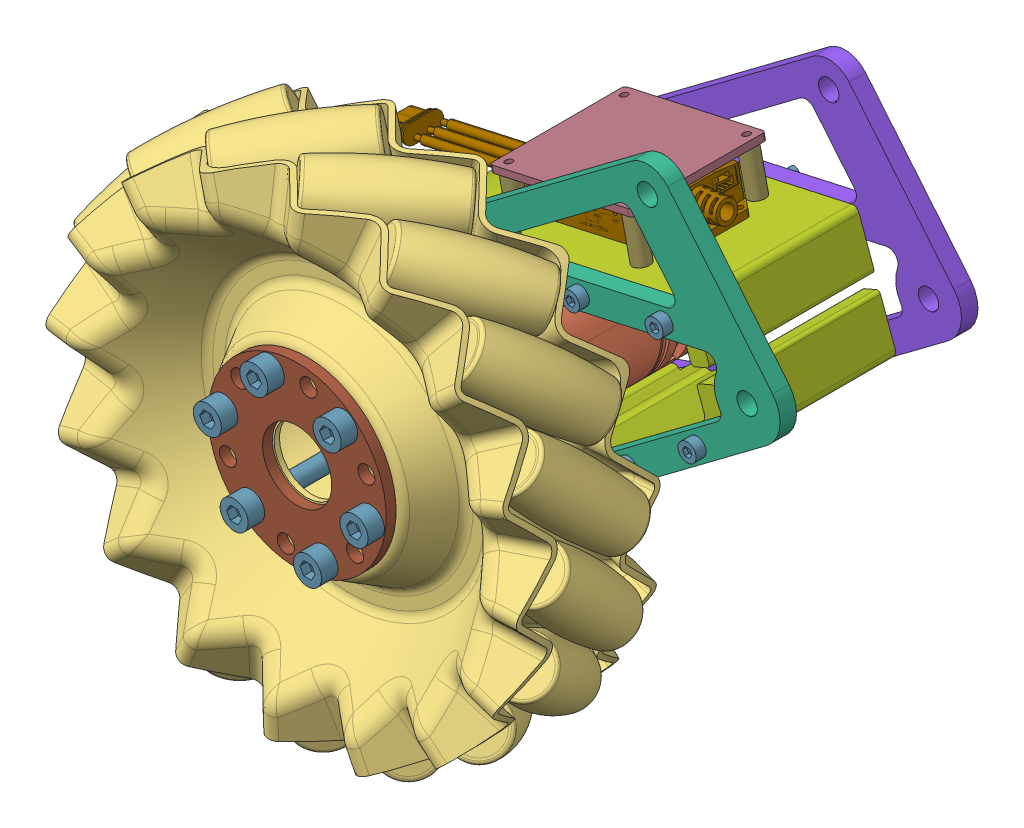
SolidWorks assembly DP_右旋轮组_1, configuration 默认. Lengths in mm.
Overall size (201.98 183.85 131.37).
38 component instances, 14 part files, 81 mates.
Components (placement in the parent):
- DP_夹紧联轴器2-1: DP_夹紧联轴器2 [默认] at (34.8209 73.9788 33.82) x (-0.925598 -0.378508 0) z (0 0 1) size (47.97 54.2 10)
- DP_RoboMaster GM3508无刷减速电机-1: DP_RoboMaster GM3508无刷减速电机 [默认] at origin size (42 44.98 98.4)
- DP_右旋_mecanum_wheel-1: DP_右旋_mecanum_wheel [默认] at (53.3369 61.5614 188.9722) x (0.971628 -0.236514 0) z (0 0 1) size (152.18 152.18 48.1)
- DP_轮组端盖_1-1: DP_轮组端盖_1 [默认] at (34.8209 73.9788 43.82) x (0.996746 -0.080602 0) z (0 0 1) size (19.5 19.5 10)
- DP_10x24x9_推力球轴承-1: DP_10x24x9_推力球轴承 [默认] at (34.8209 73.9788 28.82) x (0.526634 0.850092 0) z (0 0 1) size (24 24 10)
- DP_轮组电机安装板_1-1: DP_轮组电机安装板_1 [默认] at (122.7527 109.937 21.9) x (0.925598 0.378508 0) z (0 0 1) size (139 90.3 5)
- DP_轮组打印件垫块_1-1: DP_轮组打印件垫块_1 [默认] at (122.7527 109.937 -28.1) x (0.925598 0.378508 0) z (0 0 1) size (114.05 68 50)
- DP_轮组电机保护板_1-1: DP_轮组电机保护板_1 [默认] at (122.7527 109.937 -33.1) x (0.925598 0.378508 0) z (0 0 1) size (139 90.3 5)
- DP_C620无刷电机调速器-1: DP_C620无刷电机调速器 [默认] at (56.9242 119.261 -3.1) x (-0.976125 -0.21721 0) z (0 0 1) size (103.05 11.5 26.13)
- DP_滚花铜螺母M2x5-1: DP_滚花铜螺母M2x5 [默认] at (82.9031 114.3875 5.9) x (0.971604 0.216204 0.096132) z (-0.21721 0.976125 0) size (3 3 5)
- DP_滚花铜螺母M2x5-2: DP_滚花铜螺母M2x5 [默认] at (81.817 119.2681 -12.1) x (0.869388 0.193459 0.454684) z (0.21721 -0.976125 0) size (3 3 5)
- DP_滚花铜螺母M2x5-3: DP_滚花铜螺母M2x5 [默认] at (38.7822 104.5696 -12.1) x (0.971604 0.216204 0.096132) z (-0.21721 0.976125 0) size (3 3 5)
- DP_滚花铜螺母M2x5-4: DP_滚花铜螺母M2x5 [默认] at (37.6962 109.4502 5.9) x (-0.869388 -0.193459 -0.454684) z (0.21721 -0.976125 0) size (3 3 5)
- DP_轮毂挡板_1-1: DP_轮毂挡板_1 [默认] at (34.8209 73.9788 72.4204) x (0.93228 0.361737 0) z (0 0 1) size (54 54 3)
- DP_滚花铜螺母M2x5-5: DP_滚花铜螺母M2x5 [默认] at (41.2102 110.2322 -20.6) x (-0.869388 -0.193459 -0.454684) z (0.21721 -0.976125 0) size (3 3 5)
- DP_滚花铜螺母M2x5-6: DP_滚花铜螺母M2x5 [默认] at (79.389 113.6055 -20.6) x (-0.971604 -0.216204 -0.096132) z (-0.21721 0.976125 0) size (3 3 5)
- DP_滚花铜螺母M2x5-7: DP_滚花铜螺母M2x5 [默认] at (41.2102 110.2322 14.4) x (-0.869388 -0.193459 -0.454684) z (0.21721 -0.976125 0) size (3 3 5)
- DP_滚花铜螺母M2x5-8: DP_滚花铜螺母M2x5 [默认] at (79.389 113.6055 14.4) x (-0.971604 -0.216204 -0.096132) z (-0.21721 0.976125 0) size (3 3 5)
- DP_垫高柱-1: DP_垫高柱 [默认] at (39.7984 116.577 -20.6) x (0.92233 0.20524 0.32739) z (0.21721 -0.976125 0) size (5 5 13)
- DP_垫高柱-2: DP_垫高柱 [默认] at (76.8911 124.831 -20.6) x (0.92233 0.20524 0.32739) z (0.21721 -0.976125 0) size (5 5 13)
- DP_垫高柱-3: DP_垫高柱 [默认] at (76.8911 124.831 14.4) x (0.92233 0.20524 0.32739) z (0.21721 -0.976125 0) size (5 5 13)
- DP_垫高柱-4: DP_垫高柱 [默认] at (39.7984 116.577 14.4) x (0.92233 0.20524 0.32739) z (0.21721 -0.976125 0) size (5 5 13)
- DP_亚克力保护-1: DP_亚克力保护 [默认] at (56.4984 129.001 -3.1) x (0.976125 0.21721 0) z (0.21721 -0.976125 0) size (44 41 2)
- DP_圆柱头螺栓-1: DP_圆柱头螺栓 [M5*40] at (57.0564 70.5393 75.4204) x (1 0 0) z (0 -1 0) size (8.5 45 8.5)
- DP_圆柱头螺栓-2: DP_圆柱头螺栓 [M5*40] at (42.96 53.0025 75.4204) x (1 0 0) z (0 -1 0) size (8.5 45 8.5)
- DP_圆柱头螺栓-3: DP_圆柱头螺栓 [M5*40] at (20.7244 56.442 75.4204) x (1 0 0) z (0 -1 0) size (8.5 45 8.5)
- DP_圆柱头螺栓-4: DP_圆柱头螺栓 [M5*40] at (12.5853 77.4183 75.4204) x (1 0 0) z (0 -1 0) size (8.5 45 8.5)
- DP_圆柱头螺栓-5: DP_圆柱头螺栓 [M5*40] at (26.6818 94.9551 75.4204) x (1 0 0) z (0 -1 0) size (8.5 45 8.5)
- DP_圆柱头螺栓-6: DP_圆柱头螺栓 [M5*40] at (48.9173 91.5156 75.4204) x (1 0 0) z (0 -1 0) size (8.5 45 8.5)
- DP_圆柱头螺栓-7: DP_圆柱头螺栓 [M3*65] at (46.1761 46.2108 26.9) x (1 0 0) z (0 -1 0) size (5.5 68 5.5)
- DP_圆柱头螺栓-8: DP_圆柱头螺栓 [M3*65] at (7.0529 62.6236 26.9) x (1 0 0) z (0 -1 0) size (5.5 68 5.5)
- DP_圆柱头螺栓-9: DP_圆柱头螺栓 [M3*65] at (23.4656 101.7467 26.9) x (1 0 0) z (0 -1 0) size (5.5 68 5.5)
- DP_圆柱头螺栓-10: DP_圆柱头螺栓 [M3*65] at (46.7958 107.3773 26.9) x (1 0 0) z (0 -1 0) size (5.5 68 5.5)
- DP_圆柱头螺栓-11: DP_圆柱头螺栓 [M3*65] at (72.1751 113.0247 26.9) x (1 0 0) z (0 -1 0) size (5.5 68 5.5)
- DP_圆柱头螺栓-12: DP_圆柱头螺栓 [M3*65] at (97.5543 118.6722 26.9) x (1 0 0) z (0 -1 0) size (5.5 68 5.5)
- DP_圆柱头螺栓-13: DP_圆柱头螺栓 [M3*65] at (107.5405 91.0255 26.9) x (1 0 0) z (0 -1 0) size (5.5 68 5.5)
- DP_圆柱头螺栓-14: DP_圆柱头螺栓 [M3*65] at (86.7418 75.4238 26.9) x (1 0 0) z (0 -1 0) size (5.5 68 5.5)
- DP_圆柱头螺栓-15: DP_圆柱头螺栓 [M3*65] at (65.9431 59.8221 26.9) x (1 0 0) z (0 -1 0) size (5.5 68 5.5)
Mates (geometry in assembly coordinates):
- 同心1: concentric anti-aligned: cylinder of RoboMaster GM3508无刷减速电机-1 through (34.8209 73.9788 49.2) axis (0 0 1) radius 5; cylinder of 10x24x9_推力球轴承-1 through (34.8209 73.9788 33.82) axis (0 0 -1) radius 5
- 同心2: concentric anti-aligned: cylinder of 夹紧联轴器2-1 through (34.8209 73.9788 43.82) axis (0 0 -1) radius 5; cylinder of RoboMaster GM3508无刷减速电机-1 through (34.8209 73.9788 49.2) axis (0 0 1) radius 5
- 重合2: coincident anti-aligned: plane of 夹紧联轴器2-1 through (34.8209 73.9788 33.82) normal (0 0 -1); plane of 10x24x9_推力球轴承-1 through (34.8209 73.9788 33.82) normal (0 0 1)
- 重合3: coincident anti-aligned: plane of 夹紧联轴器2-1 through (36.0836 78.8167 43.82) normal (0.378508 -0.925598 0); plane of RoboMaster GM3508无刷减速电机-1 through (36.0836 78.8167 29.2) normal (-0.378508 0.925598 0)
- 同心3: concentric anti-aligned: cylinder of RoboMaster GM3508无刷减速电机-1 through (34.8209 73.9788 49.2) axis (0 0 1) radius 5; cylinder of DP_轮组端盖_1-1 through (34.8209 73.9788 53.82) axis (0 0 -1) radius 9.75
- 重合4: coincident anti-aligned: plane of 夹紧联轴器2-1 through (57.1527 70.8487 43.82) normal (0 0 1); plane of DP_轮组端盖_1-1 through (34.8209 73.9788 43.82) normal (0 0 -1)
- 同心4: concentric aligned: cylinder of 右旋_mecanum_wheel-1 through (34.8209 73.9788 83.494) axis (0 0 -1) radius 10; cylinder of 10x24x9_推力球轴承-1 through (34.8209 73.9788 33.82) axis (0 0 -1) radius 12
- 重合5: coincident anti-aligned: plane of 夹紧联轴器2-1 through (57.1527 70.8487 43.82) normal (0 0 1); plane of 右旋_mecanum_wheel-1 through (34.8209 73.9788 43.82) normal (0 0 -1)
- 重合6: coincident anti-aligned: plane of RoboMaster GM3508无刷减速电机-1 through (34.8209 73.9788 23.82) normal (0 0 1); plane of 10x24x9_推力球轴承-1 through (34.8209 73.9788 23.82) normal (0 0 -1)
- 同心5: concentric anti-aligned: cylinder of RoboMaster GM3508无刷减速电机-1 through (34.8209 73.9788 41.0192) axis (0 0 1) radius 21; cylinder of DP_轮组电机安装板_1-1 through (34.8209 73.9788 26.9) axis (0 0 -1) radius 13.1
- 同心6: concentric aligned: cylinder of RoboMaster GM3508无刷减速电机-1 through (51.0188 80.6027 21.9) axis (0 0 1) radius 1.65; cylinder of DP_轮组电机安装板_1-1 through (51.0188 80.6027 -7.1) axis (0 0 1) radius 2.1
- 重合8: coincident anti-aligned: plane of DP_轮组电机安装板_1-1 through (122.7527 109.937 21.9) normal (0 0 -1); plane of DP_轮组打印件垫块_1-1 through (34.8209 73.9788 21.9) normal (0 0 1)
- 同心7: concentric aligned: cylinder of RoboMaster GM3508无刷减速电机-1 through (34.8209 73.9788 -14.1) axis (0 0 -1) radius 21; cylinder of DP_轮组打印件垫块_1-1 through (34.8209 73.9788 21.9) axis (0 0 -1) radius 34
- 平行1: parallel aligned: plane of DP_轮组电机安装板_1-1 through (128.7533 101.9375 26.9) normal (0.600065 -0.799951 0); plane of DP_轮组打印件垫块_1-1 through (55.2231 46.7804 21.9) normal (0.600065 -0.799951 0)
- 同心8: concentric anti-aligned: cylinder of RoboMaster GM3508无刷减速电机-1 through (34.8209 73.9788 -16.1) axis (0 0 1) radius 21; cylinder of DP_轮组电机保护板_1-1 through (34.8209 73.9788 -28.1) axis (0 0 -1) radius 24
- 重合9: coincident anti-aligned: plane of DP_轮组打印件垫块_1-1 through (34.8209 73.9788 -28.1) normal (0 0 -1); plane of DP_轮组电机保护板_1-1 through (34.8209 73.9788 -28.1) normal (0 0 1)
- 同心9: concentric aligned: cylinder of DP_轮组电机安装板_1-1 through (92.4941 149.7417 26.9) axis (0 0 -1) radius 8; cylinder of DP_轮组电机保护板_1-1 through (92.4941 149.7417 -28.1) axis (0 0 -1) radius 8
- 重合10: coincident anti-aligned: plane of DP_轮组打印件垫块_1-1 through (27.4357 107.167 -123.4572) normal (-0.21721 0.976125 0); plane of DP_C620无刷电机调速器-1 through (59.7566 114.3592 -3.1) normal (0.21721 -0.976125 0)
- 宽度1: width anti-aligned: plane of DP_轮组电机安装板_1-1 through (122.7527 109.937 21.9) normal (0 0 -1); plane of DP_轮组电机保护板_1-1 through (34.8209 73.9788 -28.1) normal (0 0 1); plane of DP_C620无刷电机调速器-1 through (79.5499 119.7881 9.8) normal (0 0 1); plane of DP_C620无刷电机调速器-1 through (79.5499 119.7881 -16) normal (0 0 -1)
- 同心10: concentric aligned: cylinder of DP_轮组打印件垫块_1-1 through (87.0301 95.8411 5.9) axis (-0.21721 0.976125 0) radius 1.6; cylinder of DP_C620无刷电机调速器-1 through (83.8805 109.9949 5.9) axis (-0.21721 0.976125 0) radius 1
- 同心11: concentric anti-aligned: cylinder of DP_轮组打印件垫块_1-1 through (87.0301 95.8411 5.9) axis (-0.21721 0.976125 0) radius 1.6; cylinder of 滚花铜螺母M2x5-1 through (81.817 119.2681 5.9) axis (0.21721 -0.976125 0) radius 1.5
- 重合11: coincident aligned: plane of DP_轮组打印件垫块_1-1 through (27.4357 107.167 -123.4572) normal (-0.21721 0.976125 0); plane of 滚花铜螺母M2x5-1 through (81.817 119.2681 5.9) normal (-0.21721 0.976125 0)
- 同心121: concentric aligned: cylinder of DP_轮组打印件垫块_1-1 through (87.0301 95.8411 -12.1) axis (-0.21721 0.976125 0) radius 1.6; cylinder of 滚花铜螺母M2x5-2 through (81.817 119.2681 -12.1) axis (-0.21721 0.976125 0) radius 0.8
- 重合13: coincident aligned: plane of DP_轮组打印件垫块_1-1 through (27.4357 107.167 -123.4572) normal (-0.21721 0.976125 0); plane of 滚花铜螺母M2x5-2 through (81.817 119.2681 -12.1) normal (-0.21721 0.976125 0)
- 同心131: concentric anti-aligned: cylinder of DP_轮组打印件垫块_1-1 through (42.9092 86.0232 -12.1) axis (-0.21721 0.976125 0) radius 1.6; cylinder of 滚花铜螺母M2x5-3 through (37.6962 109.4502 -12.1) axis (0.21721 -0.976125 0) radius 1.5
- 重合15: coincident aligned: plane of DP_轮组打印件垫块_1-1 through (27.4357 107.167 -123.4572) normal (-0.21721 0.976125 0); plane of 滚花铜螺母M2x5-3 through (37.6962 109.4502 -12.1) normal (-0.21721 0.976125 0)
- 同心141: concentric aligned: cylinder of DP_轮组打印件垫块_1-1 through (42.9092 86.0232 5.9) axis (-0.21721 0.976125 0) radius 1.6; cylinder of 滚花铜螺母M2x5-4 through (37.6962 109.4502 5.9) axis (-0.21721 0.976125 0) radius 0.8
- 重合16: coincident aligned: plane of DP_轮组打印件垫块_1-1 through (27.4357 107.167 -123.4572) normal (-0.21721 0.976125 0); plane of 滚花铜螺母M2x5-4 through (37.6962 109.4502 5.9) normal (-0.21721 0.976125 0)
- 重合17: coincident anti-aligned: plane of 右旋_mecanum_wheel-1 through (34.8209 73.9788 72.4204) normal (0 0 1); plane of 轮毂挡板_1-1 through (34.8209 73.9788 72.4204) normal (0 0 -1)
- 同心142: concentric aligned: cylinder of 右旋_mecanum_wheel-1 through (34.8209 73.9788 83.494) axis (0 0 -1) radius 10; cylinder of 轮毂挡板_1-1 through (34.8209 73.9788 75.4204) axis (0 0 -1) radius 10.5
- 同心143: concentric anti-aligned: cylinder of 右旋_mecanum_wheel-1 through (12.5853 77.4183 72.4204) axis (0 0 1) radius 2.6; cylinder of 轮毂挡板_1-1 through (12.5853 77.4183 75.4204) axis (0 0 -1) radius 2.6
- 同心1441: concentric aligned: cylinder of DP_轮组打印件垫块_1-1 through (43.3823 100.4709 -20.6) axis (-0.21721 0.976125 0) radius 1.6; cylinder of 滚花铜螺母M2x5-5 through (41.2102 110.2322 -20.6) axis (-0.21721 0.976125 0) radius 0.8
- 重合18: coincident aligned: plane of DP_轮组打印件垫块_1-1 through (27.4357 107.167 -123.4572) normal (-0.21721 0.976125 0); plane of 滚花铜螺母M2x5-5 through (41.2102 110.2322 -20.6) normal (-0.21721 0.976125 0)
- 同心1451: concentric anti-aligned: cylinder of DP_轮组打印件垫块_1-1 through (80.4751 108.7249 -20.6) axis (-0.21721 0.976125 0) radius 1.6; cylinder of 滚花铜螺母M2x5-6 through (79.389 113.6055 -20.6) axis (0.21721 -0.976125 0) radius 0.8
- 重合21: coincident aligned: plane of DP_轮组打印件垫块_1-1 through (27.4357 107.167 -123.4572) normal (-0.21721 0.976125 0); plane of 滚花铜螺母M2x5-6 through (78.303 118.4862 -20.6) normal (-0.21721 0.976125 0)
- 同心1461: concentric aligned: cylinder of DP_轮组打印件垫块_1-1 through (43.3823 100.4709 14.4) axis (-0.21721 0.976125 0) radius 1.6; cylinder of 滚花铜螺母M2x5-7 through (41.2102 110.2322 14.4) axis (-0.21721 0.976125 0) radius 0.8
- 重合22: coincident aligned: plane of DP_轮组打印件垫块_1-1 through (27.4357 107.167 -123.4572) normal (-0.21721 0.976125 0); plane of 滚花铜螺母M2x5-7 through (41.2102 110.2322 14.4) normal (-0.21721 0.976125 0)
- 同心1471: concentric anti-aligned: cylinder of DP_轮组打印件垫块_1-1 through (80.4751 108.7249 14.4) axis (-0.21721 0.976125 0) radius 1.6; cylinder of 滚花铜螺母M2x5-8 through (78.303 118.4862 14.4) axis (0.21721 -0.976125 0) radius 1.5
- 重合25: coincident aligned: plane of DP_轮组打印件垫块_1-1 through (27.4357 107.167 -123.4572) normal (-0.21721 0.976125 0); plane of 滚花铜螺母M2x5-8 through (78.303 118.4862 14.4) normal (-0.21721 0.976125 0)
- 重合26: coincident anti-aligned: plane of DP_轮组打印件垫块_1-1 through (27.4357 107.167 -123.4572) normal (-0.21721 0.976125 0); plane of DP_垫高柱-1 through (41.2102 110.2322 -20.6) normal (0.21721 -0.976125 0)
- 同心148: concentric aligned: cylinder of 滚花铜螺母M2x5-5 through (41.2102 110.2322 -20.6) axis (-0.21721 0.976125 0) radius 0.8; cylinder of DP_垫高柱-1 through (41.2102 110.2322 -20.6) axis (-0.21721 0.976125 0) radius 2.5
- 同心1491: concentric anti-aligned: cylinder of 滚花铜螺母M2x5-6 through (78.303 118.4862 -20.6) axis (0.21721 -0.976125 0) radius 1.5; cylinder of DP_垫高柱-2 through (78.303 118.4862 -20.6) axis (-0.21721 0.976125 0) radius 2.5
- 重合271: coincident anti-aligned: plane of 滚花铜螺母M2x5-6 through (78.303 118.4862 -20.6) normal (-0.21721 0.976125 0); plane of DP_垫高柱-2 through (78.303 118.4862 -20.6) normal (0.21721 -0.976125 0)
- 同心1501: concentric aligned: cylinder of DP_轮组打印件垫块_1-1 through (80.4751 108.7249 14.4) axis (-0.21721 0.976125 0) radius 1.6; cylinder of DP_垫高柱-3 through (78.303 118.4862 14.4) axis (-0.21721 0.976125 0) radius 2.5
- 重合281: coincident anti-aligned: plane of DP_轮组打印件垫块_1-1 through (27.4357 107.167 -123.4572) normal (-0.21721 0.976125 0); plane of DP_垫高柱-3 through (78.303 118.4862 14.4) normal (0.21721 -0.976125 0)
- 同心1511: concentric aligned: cylinder of DP_轮组打印件垫块_1-1 through (43.3823 100.4709 14.4) axis (-0.21721 0.976125 0) radius 1.6; cylinder of DP_垫高柱-4 through (41.2102 110.2322 14.4) axis (-0.21721 0.976125 0) radius 2.5
- 重合291: coincident anti-aligned: plane of DP_轮组打印件垫块_1-1 through (27.4357 107.167 -123.4572) normal (-0.21721 0.976125 0); plane of DP_垫高柱-4 through (41.2102 110.2322 14.4) normal (0.21721 -0.976125 0)
- 重合30: coincident anti-aligned: plane of RoboMaster GM3508无刷减速电机-1 through (29.7918 61.9909 21.9) normal (0 0 1); plane of DP_轮组电机安装板_1-1 through (122.7527 109.937 21.9) normal (0 0 -1)
- 重合31: coincident anti-aligned: plane of DP_垫高柱-3 through (75.4792 131.1758 14.4) normal (-0.21721 0.976125 0); plane of DP_亚克力保护-1 through (56.9329 127.0488 -3.1) normal (0.21721 -0.976125 0)
- 同心152: concentric anti-aligned: cylinder of DP_垫高柱-4 through (41.2102 110.2322 14.4) axis (-0.21721 0.976125 0) radius 1.5; cylinder of DP_亚克力保护-1 through (37.9521 124.874 14.4) axis (0.21721 -0.976125 0) radius 1.1
- 同心153: concentric anti-aligned: cylinder of DP_垫高柱-1 through (41.2102 110.2322 -20.6) axis (-0.21721 0.976125 0) radius 1.5; cylinder of DP_亚克力保护-1 through (37.9521 124.874 -20.6) axis (0.21721 -0.976125 0) radius 1.1
- 同心1512: concentric anti-aligned: cylinder of DP_轮毂挡板_1-1 through (57.0564 70.5393 75.4204) axis (0 0 -1) radius 2.6; cylinder of DP_圆柱头螺栓-1 through (57.0564 70.5393 35.4204) axis (0 0 1) radius 2.5
- 重合292: coincident anti-aligned: plane of DP_轮毂挡板_1-1 through (34.8209 73.9788 75.4204) normal (0 0 1); plane of DP_圆柱头螺栓-1 through (57.0564 70.5393 75.4204) normal (0 0 -1)
- 同心15131: concentric aligned: cylinder of DP_轮毂挡板_1-1 through (42.96 53.0025 75.4204) axis (0 0 -1) radius 2.6; cylinder of DP_圆柱头螺栓-2 through (42.96 53.0025 80.4204) axis (0 0 -1) radius 4.25
- 重合2931: coincident anti-aligned: plane of DP_轮毂挡板_1-1 through (34.8209 73.9788 75.4204) normal (0 0 1); plane of DP_圆柱头螺栓-2 through (42.96 53.0025 75.4204) normal (0 0 -1)
- 同心15141: concentric aligned: cylinder of DP_轮毂挡板_1-1 through (20.7244 56.442 75.4204) axis (0 0 -1) radius 2.6; cylinder of DP_圆柱头螺栓-3 through (20.7244 56.442 80.4204) axis (0 0 -1) radius 4.25
- 重合2941: coincident anti-aligned: plane of DP_轮毂挡板_1-1 through (34.8209 73.9788 75.4204) normal (0 0 1); plane of DP_圆柱头螺栓-3 through (20.7244 56.442 75.4204) normal (0 0 -1)
- 同心15151: concentric aligned: cylinder of DP_轮毂挡板_1-1 through (12.5853 77.4183 75.4204) axis (0 0 -1) radius 2.6; cylinder of DP_圆柱头螺栓-4 through (12.5853 77.4183 80.4204) axis (0 0 -1) radius 4.25
- 重合2951: coincident anti-aligned: plane of DP_轮毂挡板_1-1 through (34.8209 73.9788 75.4204) normal (0 0 1); plane of DP_圆柱头螺栓-4 through (12.5853 77.4183 75.4204) normal (0 0 -1)
- 同心15161: concentric aligned: cylinder of DP_轮毂挡板_1-1 through (26.6818 94.9551 75.4204) axis (0 0 -1) radius 2.6; cylinder of DP_圆柱头螺栓-5 through (26.6818 94.9551 80.4204) axis (0 0 -1) radius 4.25
- 重合2961: coincident anti-aligned: plane of DP_轮毂挡板_1-1 through (34.8209 73.9788 75.4204) normal (0 0 1); plane of DP_圆柱头螺栓-5 through (26.6818 94.9551 75.4204) normal (0 0 -1)
- 同心15171: concentric aligned: cylinder of DP_轮毂挡板_1-1 through (48.9173 91.5156 75.4204) axis (0 0 -1) radius 2.6; cylinder of DP_圆柱头螺栓-6 through (48.9173 91.5156 80.4204) axis (0 0 -1) radius 4.25
- 重合2971: coincident anti-aligned: plane of DP_轮毂挡板_1-1 through (34.8209 73.9788 75.4204) normal (0 0 1); plane of DP_圆柱头螺栓-6 through (48.9173 91.5156 75.4204) normal (0 0 -1)
- 重合298: coincident anti-aligned: plane of DP_轮组电机安装板_1-1 through (122.7527 109.937 26.9) normal (0 0 1); plane of DP_圆柱头螺栓-7 through (46.1761 46.2108 26.9) normal (0 0 -1)
- 同心1518: concentric anti-aligned: cylinder of DP_轮组电机安装板_1-1 through (46.1761 46.2108 26.9) axis (0 0 -1) radius 1.6; cylinder of DP_圆柱头螺栓-7 through (46.1761 46.2108 -38.1) axis (0 0 1) radius 1.5
- 同心15191: concentric aligned: cylinder of DP_轮组电机安装板_1-1 through (7.0529 62.6236 26.9) axis (0 0 -1) radius 1.6; cylinder of DP_圆柱头螺栓-8 through (7.0529 62.6236 29.9) axis (0 0 -1) radius 2.75
- 重合2991: coincident anti-aligned: plane of DP_轮组电机安装板_1-1 through (122.7527 109.937 26.9) normal (0 0 1); plane of DP_圆柱头螺栓-8 through (7.0529 62.6236 26.9) normal (0 0 -1)
- 同心15201: concentric aligned: cylinder of DP_轮组电机安装板_1-1 through (23.4656 101.7467 26.9) axis (0 0 -1) radius 1.6; cylinder of DP_圆柱头螺栓-9 through (23.4656 101.7467 29.9) axis (0 0 -1) radius 2.75
- 重合3001: coincident anti-aligned: plane of DP_轮组电机安装板_1-1 through (122.7527 109.937 26.9) normal (0 0 1); plane of DP_圆柱头螺栓-9 through (23.4656 101.7467 26.9) normal (0 0 -1)
- 同心15211: concentric anti-aligned: cylinder of DP_轮组电机安装板_1-1 through (46.7958 107.3773 2.9) axis (0 0 1) radius 1.6; cylinder of DP_圆柱头螺栓-10 through (46.7958 107.3773 29.9) axis (0 0 -1) radius 2.75
- 重合3011: coincident anti-aligned: plane of DP_轮组电机安装板_1-1 through (122.7527 109.937 26.9) normal (0 0 1); plane of DP_圆柱头螺栓-10 through (46.7958 107.3773 26.9) normal (0 0 -1)
- 同心15221: concentric anti-aligned: cylinder of DP_轮组电机安装板_1-1 through (72.1751 113.0247 2.9) axis (0 0 1) radius 1.6; cylinder of DP_圆柱头螺栓-11 through (72.1751 113.0247 29.9) axis (0 0 -1) radius 2.75
- 重合3021: coincident anti-aligned: plane of DP_轮组电机安装板_1-1 through (122.7527 109.937 26.9) normal (0 0 1); plane of DP_圆柱头螺栓-11 through (72.1751 113.0247 26.9) normal (0 0 -1)
- 同心15231: concentric anti-aligned: cylinder of DP_轮组电机安装板_1-1 through (97.5543 118.6722 2.9) axis (0 0 1) radius 1.6; cylinder of DP_圆柱头螺栓-12 through (97.5543 118.6722 29.9) axis (0 0 -1) radius 2.75
- 重合3031: coincident anti-aligned: plane of DP_轮组电机安装板_1-1 through (122.7527 109.937 26.9) normal (0 0 1); plane of DP_圆柱头螺栓-12 through (97.5543 118.6722 26.9) normal (0 0 -1)
- 同心15241: concentric anti-aligned: cylinder of DP_轮组电机安装板_1-1 through (107.5405 91.0255 2.9) axis (0 0 1) radius 1.6; cylinder of DP_圆柱头螺栓-13 through (107.5405 91.0255 29.9) axis (0 0 -1) radius 2.75
- 重合3041: coincident anti-aligned: plane of DP_轮组电机安装板_1-1 through (122.7527 109.937 26.9) normal (0 0 1); plane of DP_圆柱头螺栓-13 through (107.5405 91.0255 26.9) normal (0 0 -1)
- 同心15251: concentric anti-aligned: cylinder of DP_轮组电机安装板_1-1 through (86.7418 75.4238 2.9) axis (0 0 1) radius 1.6; cylinder of DP_圆柱头螺栓-14 through (86.7418 75.4238 29.9) axis (0 0 -1) radius 2.75
- 重合3051: coincident anti-aligned: plane of DP_轮组电机安装板_1-1 through (122.7527 109.937 26.9) normal (0 0 1); plane of DP_圆柱头螺栓-14 through (86.7418 75.4238 26.9) normal (0 0 -1)
- 同心15261: concentric anti-aligned: cylinder of DP_轮组电机安装板_1-1 through (65.9431 59.8221 2.9) axis (0 0 1) radius 1.6; cylinder of DP_圆柱头螺栓-15 through (65.9431 59.8221 29.9) axis (0 0 -1) radius 2.75
- 重合3061: coincident anti-aligned: plane of DP_轮组电机安装板_1-1 through (122.7527 109.937 26.9) normal (0 0 1); plane of DP_圆柱头螺栓-15 through (65.9431 59.8221 26.9) normal (0 0 -1)
